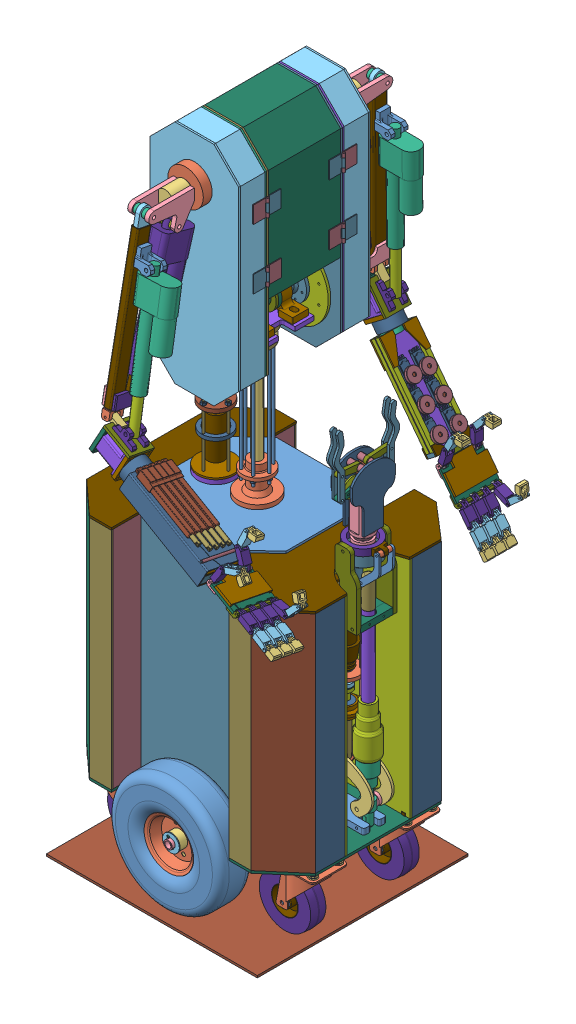
SolidWorks assembly sorbot, configuration По умолчанию. Lengths in mm.
Overall size (785.8 1577.11 772.26).
777 component instances, 239 part files, 837 mates.
Components (placement in the parent):
- wheel-1: wheel [По умолчанию] at (-13.022 1.4469 17.7637) size (270 270 80)
  - wheel.chamber-1: wheel.chamber [По умолчанию] at (6.3301 10.4899 0) size (270 270 80)
  - wheel.metal.front-1: wheel.metal.front [По умолчанию] at (6.3301 10.4899 42.7077) x (-0.311346 0.950297 0) z (0.950297 0.311346 0) size (117.48 26.95 117.48)
  - wheel.metal.internal-1: wheel.metal.internal [По умолчанию] at (6.3301 10.4899 36.3681) x (0.950297 0.311346 0) z (-0.311346 0.950297 0) size (117.48 60 117.48)
- wheel-2: wheel [По умолчанию] at (1.0599 2.4489 -290) x (-0.989924 -0.141601 0) z (0 0 -1) size (270 270 80)
  - wheel.chamber-1: wheel.chamber [По умолчанию] at (6.3301 10.4899 0) size (270 270 80)
  - wheel.metal.front-1: wheel.metal.front [По умолчанию] at (6.3301 10.4899 42.7077) x (-0.311346 0.950297 0) z (0.950297 0.311346 0) size (117.48 26.95 117.48)
  - wheel.metal.internal-1: wheel.metal.internal [По умолчанию] at (6.3301 10.4899 36.3681) x (0.950297 0.311346 0) z (-0.311346 0.950297 0) size (117.48 60 117.48)
- wheel.axis-1: wheel.axis [По умолчанию] at (-6.6918 11.9368 88.1319) x (-0.923728 -0.383049 0) z (0 0 -1) size (20 20 450)
- wheel.washer-1: wheel.washer [По умолчанию] at (-6.6918 11.9368 79.1319) size (40 40 2)
- wheel.washer-2: wheel.washer [По умолчанию] at (-6.6918 11.9368 -353.3681) size (40 40 2)
- wheel.axis.splint-1: wheel.axis.splint [По умолчанию] at (-51.8409 -4.2239 -121.73) x (0.909121 0.380793 -0.168805) z (0.181229 0.003281 0.983435) size (4.99 27.52 1.94)
- wheel.axis.splint-2: wheel.axis.splint [По умолчанию] at (-119.6931 -47.4576 -189.7376) x (-0.699932 -0.282835 -0.65582) z (0.605814 0.251217 -0.754904) size (4.99 27.52 1.94)
- wheel.disk-1: wheel.disk [По умолчанию] at (-6.6918 11.9368 -326.3681) size (86 86 70)
- gearmotor-1: gearmotor [По умолчанию] at (53.2168 119.2767 -131.0001) x (0.993251 -0.115983 0) z (0 0 1) size (79 79 282)
- wheel.bearing-1: wheel.bearing [По умолчанию] at (-6.6918 11.9368 -263.3681) x (0.993854 -0.110698 0) z (0 0 1) size (32 32 7)
- wheel.stop.bearing-2: wheel.stop.bearing [По умолчанию] at (-3.289 9.2452 -250.3457) size (52.27 52.27 14.02)
  - wheel.stop.bearing.p1-1: wheel.stop.bearing.p1 [По умолчанию] at (-3.4029 2.6916 -6.0224) size (40 40 4)
  - wheel.stop.bearing.p2-1: wheel.stop.bearing.p2 [По умолчанию] at (-3.421 17.5634 1.5621) size (7 7 7)
  - wheel.stop.bearing.p1-2: wheel.stop.bearing.p1 [По умолчанию] at (-3.4029 2.6916 8) x (-0.923728 -0.383049 0) z (0 0 -1) size (40 40 4)
  - wheel.stop.bearing.p2-3: wheel.stop.bearing.p2 [По умолчанию] at (4.0173 15.58 1.5621) x (0.866025 -0.5 0) z (0 0 1) size (7 7 7)
  - wheel.stop.bearing.p2-4: wheel.stop.bearing.p2 [По умолчанию] at (9.4674 10.1432 1.5621) x (0.5 -0.866025 0) z (0 0 1) size (7 7 7)
  - wheel.stop.bearing.p2-5: wheel.stop.bearing.p2 [По умолчанию] at (11.469 2.7097 1.5621) x (0 -1 0) z (0 0 1) size (7 7 7)
  - wheel.stop.bearing.p2-6: wheel.stop.bearing.p2 [По умолчанию] at (9.4856 -4.7286 1.5621) x (-0.5 -0.866025 0) z (0 0 1) size (7 7 7)
  - wheel.stop.bearing.p2-7: wheel.stop.bearing.p2 [По умолчанию] at (4.0488 -10.1787 1.5621) x (-0.866025 -0.5 0) z (0 0 1) size (7 7 7)
  - wheel.stop.bearing.p2-8: wheel.stop.bearing.p2 [По умолчанию] at (-3.3847 -12.1802 1.5621) x (-1 0 0) z (0 0 1) size (7 7 7)
  - wheel.stop.bearing.p2-9: wheel.stop.bearing.p2 [По умолчанию] at (-10.8231 -10.1969 1.5621) x (-0.866025 0.5 0) z (0 0 1) size (7 7 7)
  - wheel.stop.bearing.p2-10: wheel.stop.bearing.p2 [По умолчанию] at (-16.2732 -4.76 1.5621) x (-0.5 0.866025 0) z (0 0 1) size (7 7 7)
  - wheel.stop.bearing.p2-11: wheel.stop.bearing.p2 [По умолчанию] at (-18.2747 2.6734 1.5621) x (0 1 0) z (0 0 1) size (7 7 7)
  - wheel.stop.bearing.p2-12: wheel.stop.bearing.p2 [По умолчанию] at (-16.2913 10.1118 1.5621) x (0.5 0.866025 0) z (0 0 1) size (7 7 7)
  - wheel.stop.bearing.p2-13: wheel.stop.bearing.p2 [По умолчанию] at (-10.8545 15.5619 1.5621) x (0.866025 0.5 0) z (0 0 1) size (7 7 7)
- sproket.initial-1: sproket.initial [По умолчанию] at (53.2168 119.2767 -271.5001) x (0.999977 0.00678 0) z (0 0 1) size (82.09 81.83 4.4)
- gearmotor.sprocket.wheel.disk-1: gearmotor.sprocket.wheel.disk [По умолчанию] at (53.2168 119.2767 -276.8747) x (0.999997 -0.002459 0) z (0 0 1) size (68 68 28.87)
- sprocket-1: sprocket [По умолчанию] at (-6.6918 11.9368 -271.3681) size (82.09 81.83 3)
- bottom-2: bottom [По умолчанию] at (-6.1674 46.4368 -211.0406) size (543.13 5.5 438.63)
- wheel.axis.frame-3: wheel.axis.frame [По умолчанию] at (43.3082 10.4368 -242.3457) x (-1 0 0) z (0 0 1) size (126 65.5 38)
- accumulator1-1: accumulator1 [По умолчанию] at (-171.7458 53.2126 -136.828) x (0 0 -1) z (1 0 0) size (232 218.1 175)
- wheel.disk-2: wheel.disk [По умолчанию] at (-6.6918 11.9368 54.1319) x (-0.923728 -0.383049 0) z (0 0 -1) size (86 86 70)
- wheel.bearing-2: wheel.bearing [По умолчанию] at (-6.6918 11.9368 -15.8681) size (32 32 7)
- wheel.stop.bearing-3: wheel.stop.bearing [По умолчанию] at (-3.289 9.2452 -23.8681) size (52.27 52.27 14.02)
  - wheel.stop.bearing.p1-1: wheel.stop.bearing.p1 [По умолчанию] at (-3.4029 2.6916 -6.0224) size (40 40 4)
  - wheel.stop.bearing.p2-1: wheel.stop.bearing.p2 [По умолчанию] at (-3.421 17.5634 1.5621) size (7 7 7)
  - wheel.stop.bearing.p1-2: wheel.stop.bearing.p1 [По умолчанию] at (-3.4029 2.6916 8) x (-0.923728 -0.383049 0) z (0 0 -1) size (40 40 4)
  - wheel.stop.bearing.p2-3: wheel.stop.bearing.p2 [По умолчанию] at (4.0173 15.58 1.5621) x (0.866025 -0.5 0) z (0 0 1) size (7 7 7)
  - wheel.stop.bearing.p2-4: wheel.stop.bearing.p2 [По умолчанию] at (9.4674 10.1432 1.5621) x (0.5 -0.866025 0) z (0 0 1) size (7 7 7)
  - wheel.stop.bearing.p2-5: wheel.stop.bearing.p2 [По умолчанию] at (11.469 2.7097 1.5621) x (0 -1 0) z (0 0 1) size (7 7 7)
  - wheel.stop.bearing.p2-6: wheel.stop.bearing.p2 [По умолчанию] at (9.4856 -4.7286 1.5621) x (-0.5 -0.866025 0) z (0 0 1) size (7 7 7)
  - wheel.stop.bearing.p2-7: wheel.stop.bearing.p2 [По умолчанию] at (4.0488 -10.1787 1.5621) x (-0.866025 -0.5 0) z (0 0 1) size (7 7 7)
  - wheel.stop.bearing.p2-8: wheel.stop.bearing.p2 [По умолчанию] at (-3.3847 -12.1802 1.5621) x (-1 0 0) z (0 0 1) size (7 7 7)
  - wheel.stop.bearing.p2-9: wheel.stop.bearing.p2 [По умолчанию] at (-10.8231 -10.1969 1.5621) x (-0.866025 0.5 0) z (0 0 1) size (7 7 7)
  - wheel.stop.bearing.p2-10: wheel.stop.bearing.p2 [По умолчанию] at (-16.2732 -4.76 1.5621) x (-0.5 0.866025 0) z (0 0 1) size (7 7 7)
  - wheel.stop.bearing.p2-11: wheel.stop.bearing.p2 [По умолчанию] at (-18.2747 2.6734 1.5621) x (0 1 0) z (0 0 1) size (7 7 7)
  - wheel.stop.bearing.p2-12: wheel.stop.bearing.p2 [По умолчанию] at (-16.2913 10.1118 1.5621) x (0.5 0.866025 0) z (0 0 1) size (7 7 7)
  - wheel.stop.bearing.p2-13: wheel.stop.bearing.p2 [По умолчанию] at (-10.8545 15.5619 1.5621) x (0.866025 0.5 0) z (0 0 1) size (7 7 7)
- wheel.axis.frame-4: wheel.axis.frame [По умолчанию] at (-56.6918 10.4368 -29.8906) x (1 0 0) z (0 0 -1) size (126 65.5 38)
- sprocket-2: sprocket [По умолчанию] at (-6.6918 11.9368 -3.8681) x (0.99994 0.010997 0) z (0 0 1) size (82.09 81.83 3)
- gearmotor-2: gearmotor [По умолчанию] at (-40.8776 119.0545 -142.1692) x (-0.999846 -0.017524 0) z (0 0 -1) size (79 79 282)
- gearmotor.sprocket.wheel.disk-2: gearmotor.sprocket.wheel.disk [По умолчанию] at (-40.8776 119.0545 3.7054) x (-0.999846 -0.017524 0) z (0 0 -1) size (68 68 28.87)
- sproket.initial-2: sproket.initial [По умолчанию] at (-40.8776 119.0545 -1.6692) x (-0.999994 -0.003421 0) z (0 0 -1) size (82.09 81.83 4.4)
- man1-2: man1 [По умолчанию] at (221.423 424.2117 -133.5351) x (0 0 -1) z (1 0 0) size (156.5 840.47 285.01)
  - man1.actuator-1: man1.actuator [По умолчанию] at (-0.3986 -205.8789 -139.5078) x (-1 0 0) z (0 1 0.000021) size (65 65 317.39)
    - man1.drive1-1: man1.drive1 [По умолчанию] at (-4.1866 0.6029 0) size (50 50 148.25)
    - man1.drive1.frame.p1-1: man1.drive1.frame.p1 [По умолчанию] at (-4.1866 0.6029 121) size (28 28 8)
    - man1.drive1.frame.p2-1: man1.drive1.frame.p2 [По умолчанию] at (-4.1866 0.6029 121) size (65 65 8)
    - man1.drive1.frame.p4-1: man1.drive1.frame.p4 [По умолчанию] at (-4.1866 0.6029 -33) size (54 65 20)
    - man1.drive1.frame.p5-1: man1.drive1.frame.p5 [По умолчанию] at (-4.1866 0.6029 -37.3912) x (0.999995 0.003021 0) z (0 0 1) size (41.77 41.77 245)
    - man1.drive1.frame.p6-1: man1.drive1.frame.p6 [По умолчанию] at (-4.1866 0.6029 129) size (30 30 25)
    - man1.drive1.frame.p7-1: man1.drive1.frame.p7 [По умолчанию] at (-4.1866 0.6029 154) size (30 30 2)
    - man1.drive1.frame.p8-1: man1.drive1.frame.p8 [По умолчанию] at (-4.1866 0.6029 156) size (30 30 28)
    - man1.drive1.frame.p10-1: man1.drive1.frame.p10 [По умолчанию] at (-4.1866 0.6029 164) size (10.5 10.5 116)
    - man1.drive1.frame.p9-1: man1.drive1.frame.p9 [По умолчанию] at (-4.1866 0.6029 187) size (65 65 28)
    - man1.drive1.frame.p11-1: man1.drive1.frame.p11 [По умолчанию] at (-4.1866 0.6029 187) size (35 35 24)
    - man1.drive1.frame.p3-7: man1.drive1.frame.p3 [По умолчанию] at (-4.1866 0.6029 58) (suppressed, hidden)
  - man1.p1-1: man1.p1 [По умолчанию] at (52.788 -228.8789 -138.9054) x (-1 0 0) z (0 0 1) size (100 8 8)
  - man1.drive1.frame.p12-1: man1.drive1.frame.p12 [По умолчанию] at (3.788 68.5641 -138.8992) x (-1 0 0) z (0 1 0.000021) size (21 21 93)
  - man1.p2-1: man1.p2 [По умолчанию] at (-22.212 -237.9208 -123.0814) x (0 0 -1) z (-1 0 0) size (72.27 30 90)
  - man1.p5-1: man1.p5 [По умолчанию] at (4.7507 160.9388 -85.9149) x (-1 0 0) z (0 -0.002225 0.999998) size (26 90 26)
  - man1.p4-1: man1.p4 [По умолчанию] at (3.7914 125.9389 -85.9928) x (0.93549 0.000786 -0.353351) z (-0.353352 0.002082 -0.935488) size (30 487 30)
  - man1.p3-2: man1.p3 [По умолчанию] at (38.7914 154.9807 -70.1243) x (0 0 -1) z (1 0 0) size (125.25 30 85)
  - man1.p6-1: man1.p6 [По умолчанию] at (42.008 145.9388 -85.9483) x (-1 0 0) z (0 0.364371 -0.931254) size (75 8 8)
  - man1.p7-2: man1.p7 [По умолчанию] at (23.8722 69.7096 -67.4428) x (-1 0 0) z (0 -0.002225 0.999998) size (74 91.83 135.45)
  - man1.actuator-2: man1.actuator [По умолчанию] at (8.0554 58.0922 -32.4461) x (1 0 0) z (0 -0.999998 -0.002148) size (65 65 317.39)
    - man1.drive1-1: man1.drive1 [По умолчанию] at (-4.1866 0.6029 0) size (50 50 148.25)
    - man1.drive1.frame.p1-1: man1.drive1.frame.p1 [По умолчанию] at (-4.1866 0.6029 121) size (28 28 8)
    - man1.drive1.frame.p2-1: man1.drive1.frame.p2 [По умолчанию] at (-4.1866 0.6029 121) size (65 65 8)
    - man1.drive1.frame.p4-1: man1.drive1.frame.p4 [По умолчанию] at (-4.1866 0.6029 -33) size (54 65 20)
    - man1.drive1.frame.p5-1: man1.drive1.frame.p5 [По умолчанию] at (-4.1866 0.6029 -37.3912) x (0.999995 0.003021 0) z (0 0 1) size (41.77 41.77 245)
    - man1.drive1.frame.p6-1: man1.drive1.frame.p6 [По умолчанию] at (-4.1866 0.6029 129) size (30 30 25)
    - man1.drive1.frame.p7-1: man1.drive1.frame.p7 [По умолчанию] at (-4.1866 0.6029 154) size (30 30 2)
    - man1.drive1.frame.p8-1: man1.drive1.frame.p8 [По умолчанию] at (-4.1866 0.6029 156) size (30 30 28)
    - man1.drive1.frame.p10-1: man1.drive1.frame.p10 [По умолчанию] at (-4.1866 0.6029 164) size (10.5 10.5 116)
    - man1.drive1.frame.p9-1: man1.drive1.frame.p9 [По умолчанию] at (-4.1866 0.6029 187) size (65 65 28)
    - man1.drive1.frame.p11-1: man1.drive1.frame.p11 [По умолчанию] at (-4.1866 0.6029 187) size (35 35 24)
    - man1.drive1.frame.p3-7: man1.drive1.frame.p3 [По умолчанию] at (-4.1866 0.6029 58) (suppressed, hidden)
  - man1.drive1.frame.p12-2: man1.drive1.frame.p12 [По умолчанию] at (3.8689 -153.2296 -32.2971) x (1 0 0) z (0 -0.999998 -0.002148) size (21 21 93)
  - man1.p8-1: man1.p8 [По умолчанию] at (3.7914 -359.7465 -87.0735) x (0 -0.002225 0.999998) z (-1 0 0) size (145 30 54.24)
  - man1.p11-2: man1.p11 [По умолчанию] at (-11.2086 -199.8321 18.3244) x (-1 0 0) z (0 0.071625 0.997432) size (5.5 105.72 90.08)
  - man1.p12-2: man1.p12 [По умолчанию] at (-22.7871 -224.5214 -51.2659) x (1 0 0) z (0 0.19273 0.981252) size (5.5 118.7 99.86)
  - man1.p13-1: man1.p13 [По умолчанию] at (-4.1311 -234.2294 -32.471) x (1 0 0) z (0 -0.069887 -0.997555) size (7 26 26)
  - man1.p13-2: man1.p13 [По умолчанию] at (-10.2871 -314.4644 20.4089) x (1 0 0) z (0 0 1) size (7 26 26)
  - man1.p13-3: man1.p13 [По умолчанию] at (18.8689 -234.2294 -32.471) size (7 26 26)
  - man1.p12-3: man1.p12 [По умолчанию] at (24.7129 -224.5214 -51.2659) x (1 0 0) z (0 0.19273 0.981252) size (5.5 118.7 99.86)
  - man1.p13-4: man1.p13 [По умолчанию] at (24.7129 -314.4644 20.4089) x (1 0 0) z (0 -0.270753 0.962649) size (7 26 26)
  - man1.drive2-1: man1.drive2 [По умолчанию] at (3.7079 -240.2809 21.0583) x (0.972815 -0.000504 0.231584) z (0 0.999998 0.002174) size (32 32 80.98)
  - man1.p14-1: man1.p14 [По умолчанию] at (3.7079 -243.1669 21.052) x (0.999283 0.000082 -0.03786) z (0.03786 -0.002173 0.999281) size (50 191 50)
  - man1.p15-1: man1.p15 [По умолчанию] at (3.7079 -218.9022 21.1047) x (0.998805 0.000106 -0.048869) z (0.048869 -0.002172 0.998803) size (52 118 52)
  - man1.p16-1: man1.p16 [По умолчанию] at (3.7079 -152.1041 21.25) x (0.992237 0.00027 -0.124359) z (0.12436 -0.002157 0.992235) size (24.7 240 24.7)
  - man1.p17-1: man1.p17 [По умолчанию] at (3.7079 -169.2808 21.2126) x (0.999945 0.000023 -0.010535) z (0.010535 -0.002174 0.999942) size (23 37 23)
  - man1.p18-1: man1.p18 [По умолчанию] at (3.7079 -154.5438 21.2447) x (0.916473 0.00087 -0.400097) z (0.400098 -0.001993 0.91647) size (10 240 10)
  - man1.stok.2-1: man1.stok.2 [По умолчанию] at (4.7586 68.5442 21.7351) x (0.999987 -0.000011 0.005102) z (-0.005102 -0.002174 0.999985) size (31.92 103 31.92)
    - man1.p19-1: man1.p19 [По умолчанию] at (-1.0508 -2.675 0) x (1 0 -0.000645) z (0.000645 0 1) size (14 6 15.86)
    - man1.p20-1: man1.p20 [По умолчанию] at (-1.0508 -12.2265 0) x (0.999987 0 -0.005102) z (0.005102 0 0.999987) size (24 100 24)
    - man1.p19-2: man1.p19 [По умолчанию] at (-1.0508 -9.0548 0) x (1 0 -0.000645) z (0.000645 0 1) size (14 6 15.86)
    - man1.p21-1: man1.p21 [По умолчанию] at (-1.0508 -8.2265 0) x (-0.905374 0 -0.424616) z (-0.424616 0 0.905374) size (24 7 24)
  - man1.drive3-1: man1.drive3 [По умолчанию] at (3.7079 189.134 9.0302) x (-0.018472 -0.002174 0.999827) z (-0.999829 0.00004 -0.018472) size (76 103.5 76)
  - man1.p22-1: man1.p22 [По умолчанию] at (3.7079 63.509 21.7188) x (0 -0.002174 0.999998) z (-1 0 0) size (20 15 76)
  - man1.p22-2: man1.p22 [По умолчанию] at (3.7079 63.509 21.7188) x (0 0.002174 -0.999998) z (1 0 0) size (20 15 76)
  - man1.p23-1: man1.p23 [По умолчанию] at (-44.2921 93.6528 21.7843) x (1 0 0) z (0 -0.002174 0.999998) size (10 166.6 51.35)
  - man1.p24-1: man1.p24 [По умолчанию] at (3.7079 212.1339 9.0802) x (1 0 0) z (0 -0.002174 0.999998) size (76 16 76)
  - man1.p25-1: man1.p25 [По умолчанию] at (3.7079 206.1339 9.0672) x (1 0 0) z (0 -0.002174 0.999998) size (30 16 20.8)
  - man1.p26-2: man1.p26 [По умолчанию] at (-14.0001 214.8868 58.3905) x (1 0 0) z (0 -0.797207 0.603707) size (5 86.81 49.56)
  - man1.p27-1: man1.p27 [По умолчанию] at (-11.2921 220.0261 58.6688) size (10 12 12)
  - man1.p23-2: man1.p23 [По умолчанию] at (41.7079 93.6528 21.7843) x (1 0 0) z (0 -0.002174 0.999998) size (10 166.6 51.35)
  - man1.p26-3: man1.p26 [По умолчанию] at (18.7079 214.8868 58.3905) x (1 0 0) z (0 -0.797207 0.603707) size (5 86.81 49.56)
  - man1.p27-2: man1.p27 [По умолчанию] at (8.7079 220.0261 58.6688) size (10 12 12)
  - man1.p28-1: man1.p28 [По умолчанию] at (3.7079 217.1339 9.0911) x (1 0 0) z (0 -0.002174 0.999998) size (44 5 44)
  - man1.p29-1: man1.p29 [По умолчанию] at (3.7079 222.1339 9.102) x (1 0 0) z (0 -0.002174 0.999998) size (48 87 48)
  - man1.drive4-2: man1.drive4 [По умолчанию] at (3.7079 240.9454 9.1429) x (1 0 0) z (0 0.999998 0.002174) size (32 32 76.8)
  - man1.p30-1: man1.p30 [По умолчанию] at (3.7079 323.4415 9.3222) x (1 0 0) z (0 -0.002174 0.999998) size (9 22 9.04)
  - man1.p31-1: man1.p31 [По умолчанию] at (29.5403 341.472 7.7592) x (-0.97166 0.236384 0.000514) z (0 -0.002174 0.999998) size (45 45 3.2)
  - man1.p32-1: man1.p32 [По умолчанию] at (3.7079 309.2075 9.2913) x (0.999646 0.000058 -0.02662) z (0.02662 -0.002173 0.999643) size (7 52 7)
  - man1.p31-2: man1.p31 [По умолчанию] at (-22.1256 341.472 7.7592) x (0.978079 0.208235 0.000453) z (0 -0.002174 0.999998) size (45 45 3.2)
  - man1.p33-1: man1.p33 [По умолчанию] at (3.7079 357.0484 9.3953) x (1 0 -0.000001) z (0.000001 -0.002174 0.999998) size (11 4 11)
  - man1.p34-1: man1.p34 [По умолчанию] at (3.917 277.9455 29.2556) x (1 0 0) z (0 -0.002174 0.999998) size (102 143.82 5)
  - man1.p35-1: man1.p35 [По умолчанию] at (3.5428 363.0979 -0.5593) x (1 0 0) z (0 -0.002174 0.999998) size (21.92 13.34 40.06)
  - man1.p34-2: man1.p34 [По умолчанию] at (3.9108 278.1144 -15.8086) x (1 0 0) z (0 -0.002174 0.999998) size (102 143.82 5)
  - man1.p36-1: man1.p36 [По умолчанию] at (-22.1256 341.7376 -114.3921) x (-0.911615 -0.411045 -0.000894) z (-0.411046 0.911612 0.001982) size (14 12.53 14)
  - man1.p36-4: man1.p36 [По умолчанию] at (29.5403 341.2593 105.5809) x (1 0 0) z (0 0.999998 0.002174) size (14 12.53 14)
  - man1.p36-5: man1.p36 [По умолчанию] at (-22.1256 341.6777 -86.858) x (0.923728 0.383048 0.000833) z (0.383049 -0.923726 -0.002008) size (14 12.53 14)
  - man1.p36-6: man1.p36 [По умолчанию] at (29.5403 341.6777 -86.8577) x (0.923728 0.383048 0.000833) z (0.383049 -0.923726 -0.002008) size (14 12.53 14)
  - man1.p39-1: man1.p39 [По умолчанию] at (-8.83 377.6785 -10.5921) x (1 0 0) z (0 -0.002174 0.999998) size (14 14 15)
  - man1.p39-2: man1.p39 [По умолчанию] at (-8.83 377.624 14.4723) x (-0.43245 -0.901656 -0.00196) z (0 -0.002174 0.999998) size (14 14 15)
  - man1.p40-1: man1.p40 [По умолчанию] at (-55.1239 334.4334 13.8439) x (0.999874 0.01586 0.000034) z (0 -0.002174 0.999998) size (24.21 150.81 5)
  - man1.p37-2: man1.p37 [По умолчанию] at (29.5403 341.4848 1.8592) x (-0.97166 0.236384 0.000514) z (0 -0.002174 0.999998) size (47.74 16 15)
  - man1.p37-3: man1.p37 [По умолчанию] at (-22.1256 341.4848 1.8592) x (0.978079 0.208235 0.000453) z (0 -0.002174 0.999998) size (47.74 16 15)
  - man1.p38-3: man1.p38 [По умолчанию] at (-20.7759 380.2262 4.9434) x (0.937414 -0.348215 -0.000757) z (0 -0.002174 0.999998) size (59.39 24.42 8)
  - man1.p40-5: man1.p40 [По умолчанию] at (-55.1239 334.4638 -0.1561) x (0.999874 0.01586 0.000034) z (0 -0.002174 0.999998) size (24.21 150.81 5)
  - man1.p39-5: man1.p39 [По умолчанию] at (15.9138 377.6793 -10.5921) x (1 0 0) z (0 -0.002174 0.999998) size (14 14 15)
  - man1.p40-6: man1.p40 [По умолчанию] at (62.3221 333.4728 18.8418) x (-0.999874 0.01586 0.000035) z (0 0.002174 -0.999998) size (24.21 150.81 5)
  - man1.p40-7: man1.p40 [По умолчанию] at (62.3221 333.5032 4.8418) x (-0.999874 0.01586 0.000035) z (0 0.002174 -0.999998) size (24.21 150.81 5)
  - man1.p38-4: man1.p38 [По умолчанию] at (28.1311 377.9713 4.9385) x (-0.993258 0.11592 0.000252) z (0 -0.002174 0.999998) size (59.39 24.42 8)
  - man1.p39-6: man1.p39 [По умолчанию] at (15.9138 377.6248 14.4723) x (1 0 0) z (0 -0.002174 0.999998) size (14 14 15)
  - man1.p11-4: man1.p11 [По умолчанию] at (18.7914 -373.8941 -100.5086) x (1 0 0) z (0 -0.955022 0.296534) size (5.5 105.72 90.08)
- gearmotor-3: gearmotor [По умолчанию] at (-20.0648 476.1505 -136.9555) x (1 0 0) z (0 -1 0) size (79 79 282)
- wheel1-1: wheel1 [По умолчанию] at (-196.5272 -62.2972 -25.6616) x (-1 0 0) z (0 0 -1) size (200.34 170.67 200.34)
  - wheel1.p1-1: wheel1.p1 [По умолчанию] at (-12.811 1.8421 0) size (125 125 36)
  - wheel1.p2-1: wheel1.p2 [По умолчанию] at (-12.811 1.8421 0.314) size (63.07 63.07 18)
  - wheel1.p2-2: wheel1.p2 [По умолчанию] at (-12.811 1.8421 -1.8658) x (-0.923728 -0.383049 0) z (0 0 -1) size (63.07 63.07 18)
  - wheel1.p3-1: wheel1.p3 [По умолчанию] at (-12.811 1.8421 -23.186) size (26 26 45)
  - wheel1.p4-1: wheel1.p4 [По умолчанию] at (24.859 90.4164 -1.436) size (105.01 101.57 85.69)
  - wheel1.p5-1: wheel1.p5 [По умолчанию] at (-14.7105 107.5716 -31.4713) x (-0.835986 -0.053146 -0.546171) z (-0.546944 0 0.837169) size (19.35 16 19.35)
  - wheel1.p5-2: wheel1.p5 [По умолчанию] at (64.4343 107.3349 28.3568) x (-0.998587 -0.053146 0) z (0 0 1) size (19.35 16 19.35)
  - wheel1.p5-3: wheel1.p5 [По умолчанию] at (64.0198 107.4544 -30.9637) x (-0.998587 -0.053146 0) z (0 0 1) size (19.35 16 19.35)
  - wheel1.p5-4: wheel1.p5 [По умолчанию] at (-14.3812 94.4397 28.6561) x (0.835986 0.053146 0.546171) z (-0.546944 0 0.837169) size (19.35 16 19.35)
- gearmotor.fixture.p3-1: gearmotor.fixture.p3 [По умолчанию] at (-40.8776 119.0545 -206.1702) x (0.994905 -0.100817 0) z (0 0 1) size (85.63 69.7 25)
- gearmotor.fixture.p2-3: gearmotor.fixture.p2 [По умолчанию] at (10.2084 53.4933 -65.0001) size (86 101.43 182)
- gearmotor.fixture.p3-2: gearmotor.fixture.p3 [По умолчанию] at (53.2274 119.174 -90.4218) x (0.994792 -0.101924 0) z (0 0 1) size (85.63 69.7 25)
- wheel1-5: wheel1 [По умолчанию] at (187.6309 -62.2985 -24.8952) size (200.34 170.67 200.34)
  - wheel1.p1-1: wheel1.p1 [По умолчанию] at (-12.811 1.8421 0) size (125 125 36)
  - wheel1.p2-1: wheel1.p2 [По умолчанию] at (-12.811 1.8421 0.314) size (63.07 63.07 18)
  - wheel1.p2-2: wheel1.p2 [По умолчанию] at (-12.811 1.8421 -1.8658) x (-0.923728 -0.383049 0) z (0 0 -1) size (63.07 63.07 18)
  - wheel1.p3-1: wheel1.p3 [По умолчанию] at (-12.811 1.8421 -23.186) size (26 26 45)
  - wheel1.p4-1: wheel1.p4 [По умолчанию] at (24.859 90.4164 -1.436) size (105.01 101.57 85.69)
  - wheel1.p5-1: wheel1.p5 [По умолчанию] at (-14.7105 107.5716 -31.4713) x (-0.835986 -0.053146 -0.546171) z (-0.546944 0 0.837169) size (19.35 16 19.35)
  - wheel1.p5-2: wheel1.p5 [По умолчанию] at (64.4343 107.3349 28.3568) x (-0.998587 -0.053146 0) z (0 0 1) size (19.35 16 19.35)
  - wheel1.p5-3: wheel1.p5 [По умолчанию] at (64.0198 107.4544 -30.9637) x (-0.998587 -0.053146 0) z (0 0 1) size (19.35 16 19.35)
  - wheel1.p5-4: wheel1.p5 [По умолчанию] at (-14.3812 94.4397 28.6561) x (0.835986 0.053146 0.546171) z (-0.546944 0 0.837169) size (19.35 16 19.35)
- wheel1-7: wheel1 [По умолчанию] at (-196.1639 -62.2105 -250.4568) x (-1 0 0) z (0 0 -1) size (200.34 170.67 200.34)
  - wheel1.p1-1: wheel1.p1 [По умолчанию] at (-12.811 1.8421 0) size (125 125 36)
  - wheel1.p2-1: wheel1.p2 [По умолчанию] at (-12.811 1.8421 0.314) size (63.07 63.07 18)
  - wheel1.p2-2: wheel1.p2 [По умолчанию] at (-12.811 1.8421 -1.8658) x (-0.923728 -0.383049 0) z (0 0 -1) size (63.07 63.07 18)
  - wheel1.p3-1: wheel1.p3 [По умолчанию] at (-12.811 1.8421 -23.186) size (26 26 45)
  - wheel1.p4-1: wheel1.p4 [По умолчанию] at (24.859 90.4164 -1.436) size (105.01 101.57 85.69)
  - wheel1.p5-1: wheel1.p5 [По умолчанию] at (-14.7105 107.5716 -31.4713) x (-0.835986 -0.053146 -0.546171) z (-0.546944 0 0.837169) size (19.35 16 19.35)
  - wheel1.p5-2: wheel1.p5 [По умолчанию] at (64.4343 107.3349 28.3568) x (-0.998587 -0.053146 0) z (0 0 1) size (19.35 16 19.35)
  - wheel1.p5-3: wheel1.p5 [По умолчанию] at (64.0198 107.4544 -30.9637) x (-0.998587 -0.053146 0) z (0 0 1) size (19.35 16 19.35)
  - wheel1.p5-4: wheel1.p5 [По умолчанию] at (-14.3812 94.4397 28.6561) x (0.835986 0.053146 0.546171) z (-0.546944 0 0.837169) size (19.35 16 19.35)
- wheel1-8: wheel1 [По умолчанию] at (187.4476 -61.9053 -246.5204) size (200.34 170.67 200.34)
  - wheel1.p1-1: wheel1.p1 [По умолчанию] at (-12.811 1.8421 0) size (125 125 36)
  - wheel1.p2-1: wheel1.p2 [По умолчанию] at (-12.811 1.8421 0.314) size (63.07 63.07 18)
  - wheel1.p2-2: wheel1.p2 [По умолчанию] at (-12.811 1.8421 -1.8658) x (-0.923728 -0.383049 0) z (0 0 -1) size (63.07 63.07 18)
  - wheel1.p3-1: wheel1.p3 [По умолчанию] at (-12.811 1.8421 -23.186) size (26 26 45)
  - wheel1.p4-1: wheel1.p4 [По умолчанию] at (24.859 90.4164 -1.436) size (105.01 101.57 85.69)
  - wheel1.p5-1: wheel1.p5 [По умолчанию] at (-14.7105 107.5716 -31.4713) x (-0.835986 -0.053146 -0.546171) z (-0.546944 0 0.837169) size (19.35 16 19.35)
  - wheel1.p5-2: wheel1.p5 [По умолчанию] at (64.4343 107.3349 28.3568) x (-0.998587 -0.053146 0) z (0 0 1) size (19.35 16 19.35)
  - wheel1.p5-3: wheel1.p5 [По умолчанию] at (64.0198 107.4544 -30.9637) x (-0.998587 -0.053146 0) z (0 0 1) size (19.35 16 19.35)
  - wheel1.p5-4: wheel1.p5 [По умолчанию] at (-14.3812 94.4397 28.6561) x (0.835986 0.053146 0.546171) z (-0.546944 0 0.837169) size (19.35 16 19.35)
- wall1-1: wall1 [По умолчанию] at (26.1889 166.4368 -212.2424) x (0 0 1) z (-1 0 0) size (150 418.71 5)
- wall2-1: wall2 [По умолчанию] at (21.1889 166.4368 -62.2424) size (245.99 533.21 4)
- wall2-2: wall2 [По умолчанию] at (21.1889 166.4368 -216.2424) size (245.99 533.21 4)
- wall3-1: wall3 [По умолчанию] at (57.626 166.4368 -212.2424) x (0 0 1) z (-1 0 0) size (150 5 80.99)
- wall4-1: wall4 [По умолчанию] at (102.1741 112.2872 -162.1841) size (5 115 160)
- wall6-1: wall6 [По умолчанию] at (262.1742 51.9368 -58.2424) size (4 533.21 70.07)
- wall7-1: wall7 [По умолчанию] at (263.5274 51.9368 8.4769) x (0.650583 0 0.759435) z (-0.759435 0 0.650583) size (4 533.21 108.33)
- wall6-3: wall6 [По умолчанию] at (262.1742 585.1505 -216.2424) x (1 0 0) z (0 0 -1) size (4 533.21 70.07)
- wall7-3: wall7 [По умолчанию] at (182.0437 51.9368 -352.0328) x (0.650583 0 -0.759435) z (0.759435 0 0.650583) size (4 533.21 108.33)
- wall8-1: wall8 [По умолчанию] at (132.9009 51.9368 77.4522) size (52.1 533.21 4)
- wall8-2: wall8 [По умолчанию] at (132.798 585.1505 -351.1821) x (1 0 0) z (0 0 -1) size (52.1 533.21 4)
- wall9-1: wall9 [По умолчанию] at (131.9009 51.9368 18.6982) size (4 533.21 69.9)
- wall10-1: wall10 [По умолчанию] at (-1.8874 51.9368 6.1109) size (279.58 533.21 4)
- wall9-2: wall9 [По умолчанию] at (-151.6756 51.9368 18.7781) size (4 533.21 69.9)
- wall8-4: wall8 [По умолчанию] at (-146.6756 585.1505 77.4522) x (-1 0 0) z (0 0 1) size (52.1 533.21 4)
- wall7-v1-1: wall7-v1 [По умолчанию] at (-275.291 585.1505 5.6816) x (-0.67421 0 0.73854) z (0.73854 0 0.67421) size (4 533.21 104.08)
- wall11-1: wall11 [По умолчанию] at (-275.9003 51.4368 11.9312) size (4 556.08 297.39)
- wall7-v1-2: wall7-v1 [По умолчанию] at (-192.6496 585.1505 -354.9488) x (-0.67421 0 -0.73854) z (-0.73854 0 0.67421) size (4 533.21 104.08)
- wall8-5: wall8 [По умолчанию] at (-146.715 51.9368 -351.1236) x (-1 0 0) z (0 0 -1) size (52.1 533.21 4)
- wall9-3: wall9 [По умолчанию] at (-151.8245 51.9368 -341.8827) size (4 533.21 69.9)
- wall10-v1-1: wall10-v1 [По умолчанию] at (-12.0361 51.9368 -280.7872) x (-1 0 0) z (0 0 -1) size (279.58 533.21 4)
- wall9-4: wall9 [По умолчанию] at (131.7521 51.9368 -341.8827) size (4 533.21 69.9)
- cap-1: cap [По умолчанию] at (-5.7427 585.1505 -210.9644) x (0.999999 0 0.001245) z (-0.001245 0 0.999999) size (543.13 5 438.63)
- wall-fixture-v1-1: wall-fixture-v1 [По умолчанию] at (-173.7475 76.9368 76.4353) x (0 0 -1) z (1 0 0) size (22 468 22)
- wall-fixture-v2-1: wall-fixture-v2 [По умолчанию] at (-193.3747 76.9368 76.9391) size (36.03 468.21 15.37)
- wall-fixture-v2-1-1: wall-fixture-v2-1 [По умолчанию] at (-267.8225 76.9368 11.8405) x (0.73854 0 0.67421) z (-0.67421 0 0.73854) size (35.21 468.21 16.9)
- wall-fixture-v1-2: wall-fixture-v1 [По умолчанию] at (-129.6037 76.9368 8.4522) x (0 0 1) z (-1 0 0) size (22 468 22)
- wall-fixture-v2-1-2: wall-fixture-v2-1 [По умолчанию] at (-270.3872 51.4368 -279.8709) x (0 0 1) z (-1 0 0) size (35.21 468.21 16.9)
- wall-fixture-v2-2: wall-fixture-v2 [По умолчанию] at (-198.9245 51.4368 -348.5071) x (-0.738029 0 0.674769) z (-0.674769 0 -0.738029) size (36.03 468.21 15.37)
- wall-fixture-v1-3: wall-fixture-v1 [По умолчанию] at (-152.8245 51.4368 -329.0518) x (-1 0 0) z (0 0 -1) size (22 468 22)
- wall-fixture-v1-4: wall-fixture-v1 [По умолчанию] at (-150.8245 51.4368 -303.2005) size (22 468 22)
- wall-fixture-v1-5: wall-fixture-v1 [По умолчанию] at (115.6802 51.4368 -282.1286) x (0 0 -1) z (1 0 0) size (22 468 22)
- wall-fixture-v1-6: wall-fixture-v1 [По умолчанию] at (159.8239 51.4368 -350.1821) x (0 0 1) z (-1 0 0) size (22 468 22)
- wall-fixture-v2-2-1: wall-fixture-v2-2 [По умолчанию] at (179.7171 51.4368 -350.669) x (-1 0 0) z (0 0 -1) size (37.63 460 15.83)
- wall-fixture-v2-3-1: wall-fixture-v2-3 [По умолчанию] at (259.0363 51.4368 -285.4128) x (-0.759435 0 -0.650583) z (0.650583 0 -0.759435) size (34.89 460 17.21)
- wall-fixture-v1-7: wall-fixture-v1 [По умолчанию] at (240.1022 51.4368 -218.2424) x (0 0 -1) z (1 0 0) size (22 468 22)
- wall-fixture-v1-8: wall-fixture-v1 [По умолчанию] at (261.1742 51.4368 -35.1705) x (-1 0 0) z (0 0 -1) size (22 468 22)
- wall-fixture-v2-4-1: wall-fixture-v2-4 [По умолчанию] at (259.1218 591.4368 11.3719) x (-0.758224 0 0.651995) z (0.651995 0 0.758224) size (34.89 460 17.21)
- wall-fixture-v2-5-1: wall-fixture-v2-5 [По умолчанию] at (178.2705 591.4368 76.9391) x (-1 0 0) z (0 0 1) size (37.63 460 15.83)
- wall-fixture-v1-9: wall-fixture-v1 [По умолчанию] at (138.9009 51.4368 55.3804) size (22 468 22)
- wall-fixture-v1-10: wall-fixture-v1 [По умолчанию] at (136.9009 76.9368 29.5241) x (-1 0 0) z (0 0 -1) size (22 468 22)
- wall-fixture-6-1: wall-fixture-6 [По умолчанию] at (79.1022 164.4368 -79.0844) x (0 -1 0) z (1 0 0) size (22 116 22)
- wall-fixture-6-2: wall-fixture-6 [По умолчанию] at (21.1889 187.5087 -195.3202) x (1 0 0) z (0 -1 0) size (22 116 22)
- wall-fixture-7-1: wall-fixture-7 [По умолчанию] at (21.2432 187.5087 -58.2424) x (0 0 -1) z (0 -1 0) size (22 81 22)
- wall-fixture-7-2: wall-fixture-7 [По умолчанию] at (102.2155 187.5087 -216.2424) x (0 0 1) z (0 -1 0) size (22 81 22)
- wall-fixture-8-1: wall-fixture-8 [По умолчанию] at (123.2459 51.3998 -216.2424) x (0 0 1) z (-1 0 0) size (22 112 22)
- wall-fixture-8-2: wall-fixture-8 [По умолчанию] at (102.1741 51.9112 -79.3142) size (22 112 22)
- wall-fixture-9-1: wall-fixture-9 [По умолчанию] at (21.1889 187.3953 -79.3142) size (22 390 22)
- wall-fixture-9-2: wall-fixture-9 [По умолчанию] at (42.2608 187.5289 -216.2424) x (0 0 1) z (-1 0 0) size (22 390 22)
- turret-1: turret [По умолчанию] at (-28.0267 628.2367 -136.0551) x (0.993667 0 -0.112365) z (0.112365 0 0.993667) size (200 17.64 200)
  - turret-p1-1: turret-p1 [По умолчанию] at (8.0127 -33.0433 0) size (180 12.6 180)
  - turret-p2-1: turret-p2 [По умолчанию] at (70.5799 -32.9814 -33.6477) size (10 10 10)
  - turret-p2-2: turret-p2 [По умолчанию] at (54.1999 -32.9814 -53.9774) x (0.932472 0 -0.361242) z (0.361242 0 0.932472) size (10 10 10)
  - turret-p2-3: turret-p2 [По умолчанию] at (31.5821 -32.9814 -67.0172) x (0.739009 0 -0.673696) z (0.673696 0 0.739009) size (10 10 10)
  - turret-p2-4: turret-p2 [По умолчанию] at (5.7811 -32.9814 -71.0059) x (0.445738 0 -0.895163) z (0.895163 0 0.445738) size (10 10 10)
  - turret-p2-5: turret-p2 [По умолчанию] at (-19.7185 -32.9814 -65.4049) x (0.092268 0 -0.995734) z (0.995734 0 0.092268) size (10 10 10)
  - turret-p2-6: turret-p2 [По умолчанию] at (-41.4728 -32.9814 -50.9706) x (-0.273663 0 -0.961826) z (0.961826 0 -0.273663) size (10 10 10)
  - turret-p2-7: turret-p2 [По умолчанию] at (-56.5439 -32.9814 -29.6524) x (-0.602635 0 -0.798017) z (0.798017 0 -0.602635) size (10 10 10)
  - turret-p2-8: turret-p2 [По умолчанию] at (-62.8962 -32.9814 -4.3296) x (-0.850217 0 -0.526432) z (0.526432 0 -0.850217) size (10 10 10)
  - turret-p2-9: turret-p2 [По умолчанию] at (-59.6719 -32.9814 21.5781) x (-0.982973 0 -0.18375) z (0.18375 0 -0.982973) size (10 10 10)
  - turret-p2-10: turret-p2 [По умолчанию] at (-47.3064 -32.9814 44.5714) x (-0.982973 0 0.18375) z (-0.18375 0 -0.982973) size (10 10 10)
  - turret-p2-11: turret-p2 [По умолчанию] at (-27.4698 -32.9814 61.5452) x (-0.850217 0 0.526432) z (-0.526432 0 -0.850217) size (10 10 10)
  - turret-p2-12: turret-p2 [По умолчанию] at (-2.8411 -32.9814 70.2069) x (-0.602635 0 0.798017) z (-0.798017 0 -0.602635) size (10 10 10)
  - turret-p2-13: turret-p2 [По умолчанию] at (23.2535 -32.9814 69.3868) x (-0.273663 0 0.961826) z (-0.961826 0 -0.273663) size (10 10 10)
  - turret-p2-14: turret-p2 [По умолчанию] at (47.2898 -32.9814 59.1957) x (0.092268 0 0.995734) z (-0.995734 0 0.092268) size (10 10 10)
  - turret-p2-15: turret-p2 [По умолчанию] at (66.0214 -32.9814 41.0098) x (0.445738 0 0.895163) z (-0.895163 0 0.445738) size (10 10 10)
  - turret-p2-16: turret-p2 [По умолчанию] at (76.9187 -32.9814 17.2853) x (0.739009 0 0.673696) z (-0.673696 0 0.739009) size (10 10 10)
  - turret-p2-17: turret-p2 [По умолчанию] at (78.5098 -32.9814 -8.7736) x (0.932472 0 0.361242) z (-0.361242 0 0.932472) size (10 10 10)
  - turret-p3-1: turret-p3 [По умолчанию] at (8.0127 -35.0433 0) x (0.999999 0 0.001108) z (-0.001108 0 0.999999) size (180 2 180)
  - turret-p5-1: turret-p5 [По умолчанию] at (92.4476 -23.6726 -1.2982) size (3 3 3)
  - turret-p5-2: turret-p5 [По умолчанию] at (92.1994 -23.6726 -6.5974) x (0.998027 0 -0.062791) z (0.062791 0 0.998027) size (3 3 3)
  - turret-p5-3: turret-p5 [По умолчанию] at (91.6191 -23.6726 -11.8705) x (0.992115 0 -0.125333) z (0.125333 0 0.992115) size (3 3 3)
  - turret-p5-4: turret-p5 [По умолчанию] at (90.7087 -23.6726 -17.0968) x (0.982287 0 -0.187381) z (0.187381 0 0.982287) size (3 3 3)
  - turret-p5-5: turret-p5 [По умолчанию] at (89.472 -23.6726 -22.2556) x (0.968583 0 -0.24869) z (0.24869 0 0.968583) size (3 3 3)
  - turret-p5-6: turret-p5 [По умолчанию] at (87.9138 -23.6726 -27.3265) x (0.951057 0 -0.309017) z (0.309017 0 0.951057) size (3 3 3)
  - turret-p5-7: turret-p5 [По умолчанию] at (86.0403 -23.6726 -32.2896) x (0.929776 0 -0.368125) z (0.368125 0 0.929776) size (3 3 3)
  - turret-p5-8: turret-p5 [По умолчанию] at (83.8589 -23.6726 -37.1253) x (0.904827 0 -0.425779) z (0.425779 0 0.904827) size (3 3 3)
  - turret-p5-9: turret-p5 [По умолчанию] at (81.3781 -23.6726 -41.8145) x (0.876307 0 -0.481754) z (0.481754 0 0.876307) size (3 3 3)
  - turret-p5-10: turret-p5 [По умолчанию] at (78.6078 -23.6726 -46.3386) x (0.844328 0 -0.535827) z (0.535827 0 0.844328) size (3 3 3)
  - turret-p5-11: turret-p5 [По умолчанию] at (75.5589 -23.6726 -50.6799) x (0.809017 0 -0.587785) z (0.587785 0 0.809017) size (3 3 3)
  - turret-p5-12: turret-p5 [По умолчанию] at (72.2433 -23.6726 -54.8211) x (0.770513 0 -0.637424) z (0.637424 0 0.770513) size (3 3 3)
  - turret-p5-13: turret-p5 [По умолчанию] at (68.6744 -23.6726 -58.746) x (0.728969 0 -0.684547) z (0.684547 0 0.728969) size (3 3 3)
  - turret-p5-14: turret-p5 [По умолчанию] at (64.866 -23.6726 -62.4391) x (0.684547 0 -0.728969) z (0.728969 0 0.684547) size (3 3 3)
  - turret-p5-15: turret-p5 [По умолчанию] at (60.8332 -23.6726 -65.8857) x (0.637424 0 -0.770513) z (0.770513 0 0.637424) size (3 3 3)
  - turret-p5-16: turret-p5 [По умолчанию] at (56.592 -23.6726 -69.0723) x (0.587785 0 -0.809017) z (0.809017 0 0.587785) size (3 3 3)
  - turret-p5-17: turret-p5 [По умолчанию] at (52.159 -23.6726 -71.9864) x (0.535827 0 -0.844328) z (0.844328 0 0.535827) size (3 3 3)
  - turret-p5-18: turret-p5 [По умолчанию] at (47.5518 -23.6726 -74.6163) x (0.481754 0 -0.876307) z (0.876307 0 0.481754) size (3 3 3)
  - turret-p5-19: turret-p5 [По умолчанию] at (42.7886 -23.6726 -76.9517) x (0.425779 0 -0.904827) z (0.904827 0 0.425779) size (3 3 3)
  - turret-p5-20: turret-p5 [По умолчанию] at (37.8882 -23.6726 -78.9835) x (0.368125 0 -0.929776) z (0.929776 0 0.368125) size (3 3 3)
  - turret-p5-21: turret-p5 [По умолчанию] at (32.8698 -23.6726 -80.7035) x (0.309017 0 -0.951057) z (0.951057 0 0.309017) size (3 3 3)
  - turret-p5-22: turret-p5 [По умолчанию] at (27.7533 -23.6726 -82.1051) x (0.24869 0 -0.968583) z (0.968583 0 0.24869) size (3 3 3)
  - turret-p5-23: turret-p5 [По умолчанию] at (22.559 -23.6726 -83.1826) x (0.187381 0 -0.982287) z (0.982287 0 0.187381) size (3 3 3)
  - turret-p5-24: turret-p5 [По умолчанию] at (17.3072 -23.6726 -83.9318) x (0.125333 0 -0.992115) z (0.992115 0 0.125333) size (3 3 3)
  - turret-p5-25: turret-p5 [По умолчанию] at (12.0187 -23.6726 -84.3498) x (0.062791 0 -0.998027) z (0.998027 0 0.062791) size (3 3 3)
  - turret-p5-26: turret-p5 [По умолчанию] at (6.7144 -23.6726 -84.4349) x (0 0 -1) z (1 0 0) size (3 3 3)
  - turret-p5-27: turret-p5 [По умолчанию] at (1.4153 -23.6726 -84.1868) x (-0.062791 0 -0.998027) z (0.998027 0 -0.062791) size (3 3 3)
  - turret-p5-28: turret-p5 [По умолчанию] at (-3.8578 -23.6726 -83.6064) x (-0.125333 0 -0.992115) z (0.992115 0 -0.125333) size (3 3 3)
  - turret-p5-29: turret-p5 [По умолчанию] at (-9.0841 -23.6726 -82.696) x (-0.187381 0 -0.982287) z (0.982287 0 -0.187381) size (3 3 3)
  - turret-p5-30: turret-p5 [По умолчанию] at (-14.2429 -23.6726 -81.4594) x (-0.24869 0 -0.968583) z (0.968583 0 -0.24869) size (3 3 3)
  - turret-p5-31: turret-p5 [По умолчанию] at (-19.3138 -23.6726 -79.9012) x (-0.309017 0 -0.951057) z (0.951057 0 -0.309017) size (3 3 3)
  - turret-p5-32: turret-p5 [По умолчанию] at (-24.2769 -23.6726 -78.0277) x (-0.368125 0 -0.929776) z (0.929776 0 -0.368125) size (3 3 3)
  - turret-p5-33: turret-p5 [По умолчанию] at (-29.1126 -23.6726 -75.8462) x (-0.425779 0 -0.904827) z (0.904827 0 -0.425779) size (3 3 3)
  - turret-p5-34: turret-p5 [По умолчанию] at (-33.8018 -23.6726 -73.3654) x (-0.481754 0 -0.876307) z (0.876307 0 -0.481754) size (3 3 3)
  - turret-p5-35: turret-p5 [По умолчанию] at (-38.3259 -23.6726 -70.5951) x (-0.535827 0 -0.844328) z (0.844328 0 -0.535827) size (3 3 3)
  - turret-p5-36: turret-p5 [По умолчанию] at (-42.6672 -23.6726 -67.5462) x (-0.587785 0 -0.809017) z (0.809017 0 -0.587785) size (3 3 3)
  - turret-p5-37: turret-p5 [По умолчанию] at (-46.8085 -23.6726 -64.2307) x (-0.637424 0 -0.770513) z (0.770513 0 -0.637424) size (3 3 3)
  - turret-p5-38: turret-p5 [По умолчанию] at (-50.7334 -23.6726 -60.6617) x (-0.684547 0 -0.728969) z (0.728969 0 -0.684547) size (3 3 3)
  - turret-p5-39: turret-p5 [По умолчанию] at (-54.4264 -23.6726 -56.8533) x (-0.728969 0 -0.684547) z (0.684547 0 -0.728969) size (3 3 3)
  - turret-p5-40: turret-p5 [По умолчанию] at (-57.873 -23.6726 -52.8205) x (-0.770513 0 -0.637424) z (0.637424 0 -0.770513) size (3 3 3)
  - turret-p5-41: turret-p5 [По умолчанию] at (-61.0597 -23.6726 -48.5793) x (-0.809017 0 -0.587785) z (0.587785 0 -0.809017) size (3 3 3)
  - turret-p5-42: turret-p5 [По умолчанию] at (-63.9737 -23.6726 -44.1463) x (-0.844328 0 -0.535827) z (0.535827 0 -0.844328) size (3 3 3)
  - turret-p5-43: turret-p5 [По умолчанию] at (-66.6036 -23.6726 -39.5392) x (-0.876307 0 -0.481754) z (0.481754 0 -0.876307) size (3 3 3)
  - turret-p5-44: turret-p5 [По умолчанию] at (-68.9391 -23.6726 -34.7759) x (-0.904827 0 -0.425779) z (0.425779 0 -0.904827) size (3 3 3)
  - turret-p5-45: turret-p5 [По умолчанию] at (-70.9708 -23.6726 -29.8755) x (-0.929776 0 -0.368125) z (0.368125 0 -0.929776) size (3 3 3)
  - turret-p5-46: turret-p5 [По умолчанию] at (-72.6908 -23.6726 -24.8571) x (-0.951057 0 -0.309017) z (0.309017 0 -0.951057) size (3 3 3)
  - turret-p5-47: turret-p5 [По умолчанию] at (-74.0924 -23.6726 -19.7407) x (-0.968583 0 -0.24869) z (0.24869 0 -0.968583) size (3 3 3)
  - turret-p5-48: turret-p5 [По умолчанию] at (-75.1699 -23.6726 -14.5463) x (-0.982287 0 -0.187381) z (0.187381 0 -0.982287) size (3 3 3)
  - turret-p5-49: turret-p5 [По умолчанию] at (-75.9191 -23.6726 -9.2945) x (-0.992115 0 -0.125333) z (0.125333 0 -0.992115) size (3 3 3)
  - turret-p5-50: turret-p5 [По умолчанию] at (-76.3371 -23.6726 -4.006) x (-0.998027 0 -0.062791) z (0.062791 0 -0.998027) size (3 3 3)
  - turret-p5-51: turret-p5 [По умолчанию] at (-76.4222 -23.6726 1.2982) x (-1 0 0) z (0 0 -1) size (3 3 3)
  - turret-p5-52: turret-p5 [По умолчанию] at (-76.1741 -23.6726 6.5974) x (-0.998027 0 0.062791) z (-0.062791 0 -0.998027) size (3 3 3)
  - turret-p5-53: turret-p5 [По умолчанию] at (-75.5937 -23.6726 11.8705) x (-0.992115 0 0.125333) z (-0.125333 0 -0.992115) size (3 3 3)
  - turret-p5-54: turret-p5 [По умолчанию] at (-74.6834 -23.6726 17.0968) x (-0.982287 0 0.187381) z (-0.187381 0 -0.982287) size (3 3 3)
  - turret-p5-55: turret-p5 [По умолчанию] at (-73.4467 -23.6726 22.2556) x (-0.968583 0 0.24869) z (-0.24869 0 -0.968583) size (3 3 3)
  - turret-p5-56: turret-p5 [По умолчанию] at (-71.8885 -23.6726 27.3265) x (-0.951057 0 0.309017) z (-0.309017 0 -0.951057) size (3 3 3)
  - turret-p5-57: turret-p5 [По умолчанию] at (-70.015 -23.6726 32.2896) x (-0.929776 0 0.368125) z (-0.368125 0 -0.929776) size (3 3 3)
  - turret-p5-58: turret-p5 [По умолчанию] at (-67.8335 -23.6726 37.1253) x (-0.904827 0 0.425779) z (-0.425779 0 -0.904827) size (3 3 3)
  - turret-p5-59: turret-p5 [По умолчанию] at (-65.3527 -23.6726 41.8145) x (-0.876307 0 0.481754) z (-0.481754 0 -0.876307) size (3 3 3)
  - turret-p5-60: turret-p5 [По умолчанию] at (-62.5824 -23.6726 46.3386) x (-0.844328 0 0.535827) z (-0.535827 0 -0.844328) size (3 3 3)
  - turret-p5-61: turret-p5 [По умолчанию] at (-59.5335 -23.6726 50.6799) x (-0.809017 0 0.587785) z (-0.587785 0 -0.809017) size (3 3 3)
  - turret-p5-62: turret-p5 [По умолчанию] at (-56.218 -23.6726 54.8211) x (-0.770513 0 0.637424) z (-0.637424 0 -0.770513) size (3 3 3)
  - turret-p5-63: turret-p5 [По умолчанию] at (-52.649 -23.6726 58.746) x (-0.728969 0 0.684547) z (-0.684547 0 -0.728969) size (3 3 3)
  - turret-p5-64: turret-p5 [По умолчанию] at (-48.8406 -23.6726 62.4391) x (-0.684547 0 0.728969) z (-0.728969 0 -0.684547) size (3 3 3)
  - turret-p5-65: turret-p5 [По умолчанию] at (-44.8078 -23.6726 65.8857) x (-0.637424 0 0.770513) z (-0.770513 0 -0.637424) size (3 3 3)
  - turret-p5-66: turret-p5 [По умолчанию] at (-40.5666 -23.6726 69.0723) x (-0.587785 0 0.809017) z (-0.809017 0 -0.587785) size (3 3 3)
  - turret-p5-67: turret-p5 [По умолчанию] at (-36.1337 -23.6726 71.9864) x (-0.535827 0 0.844328) z (-0.844328 0 -0.535827) size (3 3 3)
  - turret-p5-68: turret-p5 [По умолчанию] at (-31.5265 -23.6726 74.6163) x (-0.481754 0 0.876307) z (-0.876307 0 -0.481754) size (3 3 3)
  - turret-p5-69: turret-p5 [По умолчанию] at (-26.7633 -23.6726 76.9517) x (-0.425779 0 0.904827) z (-0.904827 0 -0.425779) size (3 3 3)
  - turret-p5-70: turret-p5 [По умолчанию] at (-21.8628 -23.6726 78.9835) x (-0.368125 0 0.929776) z (-0.929776 0 -0.368125) size (3 3 3)
  - turret-p5-71: turret-p5 [По умолчанию] at (-16.8444 -23.6726 80.7035) x (-0.309017 0 0.951057) z (-0.951057 0 -0.309017) size (3 3 3)
  - turret-p5-72: turret-p5 [По умолчанию] at (-11.728 -23.6726 82.1051) x (-0.24869 0 0.968583) z (-0.968583 0 -0.24869) size (3 3 3)
  - turret-p5-73: turret-p5 [По умолчанию] at (-6.5336 -23.6726 83.1826) x (-0.187381 0 0.982287) z (-0.982287 0 -0.187381) size (3 3 3)
  - turret-p5-74: turret-p5 [По умолчанию] at (-1.2818 -23.6726 83.9318) x (-0.125333 0 0.992115) z (-0.992115 0 -0.125333) size (3 3 3)
  - turret-p5-75: turret-p5 [По умолчанию] at (4.0066 -23.6726 84.3498) x (-0.062791 0 0.998027) z (-0.998027 0 -0.062791) size (3 3 3)
  - turret-p5-76: turret-p5 [По умолчанию] at (9.3109 -23.6726 84.4349) x (0 0 1) z (-1 0 0) size (3 3 3)
  - turret-p5-77: turret-p5 [По умолчанию] at (14.6101 -23.6726 84.1868) x (0.062791 0 0.998027) z (-0.998027 0 0.062791) size (3 3 3)
  - turret-p5-78: turret-p5 [По умолчанию] at (19.8832 -23.6726 83.6064) x (0.125333 0 0.992115) z (-0.992115 0 0.125333) size (3 3 3)
  - turret-p5-79: turret-p5 [По умолчанию] at (25.1094 -23.6726 82.696) x (0.187381 0 0.982287) z (-0.982287 0 0.187381) size (3 3 3)
  - turret-p5-80: turret-p5 [По умолчанию] at (30.2682 -23.6726 81.4594) x (0.24869 0 0.968583) z (-0.968583 0 0.24869) size (3 3 3)
  - turret-p5-81: turret-p5 [По умолчанию] at (35.3392 -23.6726 79.9012) x (0.309017 0 0.951057) z (-0.951057 0 0.309017) size (3 3 3)
  - turret-p5-82: turret-p5 [По умолчанию] at (40.3023 -23.6726 78.0277) x (0.368125 0 0.929776) z (-0.929776 0 0.368125) size (3 3 3)
  - turret-p5-83: turret-p5 [По умолчанию] at (45.138 -23.6726 75.8462) x (0.425779 0 0.904827) z (-0.904827 0 0.425779) size (3 3 3)
  - turret-p5-84: turret-p5 [По умолчанию] at (49.8271 -23.6726 73.3654) x (0.481754 0 0.876307) z (-0.876307 0 0.481754) size (3 3 3)
  - turret-p5-85: turret-p5 [По умолчанию] at (54.3513 -23.6726 70.5951) x (0.535827 0 0.844328) z (-0.844328 0 0.535827) size (3 3 3)
  - turret-p4-1: turret-p4 [По умолчанию] at (8.6103 -37.0862 -3.1032) size (200 17 200)
  - turret-p5-86: turret-p5 [По умолчанию] at (58.6926 -23.6726 67.5462) x (0.587785 0 0.809017) z (-0.809017 0 0.587785) size (3 3 3)
  - turret-p5-87: turret-p5 [По умолчанию] at (62.8338 -23.6726 64.2307) x (0.637424 0 0.770513) z (-0.770513 0 0.637424) size (3 3 3)
  - turret-p5-88: turret-p5 [По умолчанию] at (66.7587 -23.6726 60.6617) x (0.684547 0 0.728969) z (-0.728969 0 0.684547) size (3 3 3)
  - turret-p5-89: turret-p5 [По умолчанию] at (70.4518 -23.6726 56.8533) x (0.728969 0 0.684547) z (-0.684547 0 0.728969) size (3 3 3)
  - turret-p5-90: turret-p5 [По умолчанию] at (73.8984 -23.6726 52.8205) x (0.770513 0 0.637424) z (-0.637424 0 0.770513) size (3 3 3)
  - turret-p5-91: turret-p5 [По умолчанию] at (77.085 -23.6726 48.5793) x (0.809017 0 0.587785) z (-0.587785 0 0.809017) size (3 3 3)
  - turret-p5-92: turret-p5 [По умолчанию] at (79.999 -23.6726 44.1463) x (0.844328 0 0.535827) z (-0.535827 0 0.844328) size (3 3 3)
  - turret-p5-93: turret-p5 [По умолчанию] at (82.629 -23.6726 39.5392) x (0.876307 0 0.481754) z (-0.481754 0 0.876307) size (3 3 3)
  - turret-p5-94: turret-p5 [По умолчанию] at (84.9644 -23.6726 34.7759) x (0.904827 0 0.425779) z (-0.425779 0 0.904827) size (3 3 3)
  - turret-p5-95: turret-p5 [По умолчанию] at (86.9962 -23.6726 29.8755) x (0.929776 0 0.368125) z (-0.368125 0 0.929776) size (3 3 3)
  - turret-p5-96: turret-p5 [По умолчанию] at (88.7162 -23.6726 24.8571) x (0.951057 0 0.309017) z (-0.309017 0 0.951057) size (3 3 3)
  - turret-p5-97: turret-p5 [По умолчанию] at (90.1177 -23.6726 19.7407) x (0.968583 0 0.24869) z (-0.24869 0 0.968583) size (3 3 3)
  - turret-p5-98: turret-p5 [По умолчанию] at (91.1953 -23.6726 14.5463) x (0.982287 0 0.187381) z (-0.187381 0 0.982287) size (3 3 3)
  - turret-p5-99: turret-p5 [По умолчанию] at (91.9445 -23.6726 9.2945) x (0.992115 0 0.125333) z (-0.125333 0 0.992115) size (3 3 3)
  - turret-p5-100: turret-p5 [По умолчанию] at (92.3625 -23.6726 4.006) x (0.998027 0 0.062791) z (-0.062791 0 0.998027) size (3 3 3)
- bolt1-1: bolt1 [По умолчанию] at (252.2608 28.1179 -56.3731) x (0 0 1) z (1 0 0) size (14 40.5 16.17)
- bolt1-2: bolt1 [По умолчанию] at (172.9115 28.0264 3.3236) x (0 0 1) z (1 0 0) size (14 40.5 16.17)
- bolt1-3: bolt1 [По умолчанию] at (251.9125 28.1164 3.3175) x (0 0 1) z (1 0 0) size (14 40.5 16.17)
- bolt1-4: bolt1 [По умолчанию] at (172.9018 28.0211 -56.2899) x (0 0 1) z (1 0 0) size (14 40.5 16.17)
- bolt1-5: bolt1 [По умолчанию] at (172.7717 28.5111 -218.0055) x (0.546944 0 -0.837169) z (-0.837169 0 -0.546944) size (14 40.5 16.17)
- bolt1-6: bolt1 [По умолчанию] at (251.718 28.5111 -277.7613) x (0.546944 0 -0.837169) z (-0.837169 0 -0.546944) size (14 40.5 16.17)
- bolt1-7: bolt1 [По умолчанию] at (172.7558 28.5111 -277.7529) x (0.546944 0 -0.837169) z (-0.837169 0 -0.546944) size (14 40.5 16.17)
- bolt1-8: bolt1 [По умолчанию] at (251.8056 28.5111 -218.1439) x (0.546944 0 -0.837169) z (-0.837169 0 -0.546944) size (14 40.5 16.17)
- bolt1-9: bolt1 [По умолчанию] at (-260.5376 28.2059 -219.1987) x (0.546944 0 -0.837169) z (-0.837169 0 -0.546944) size (14 40.5 16.17)
